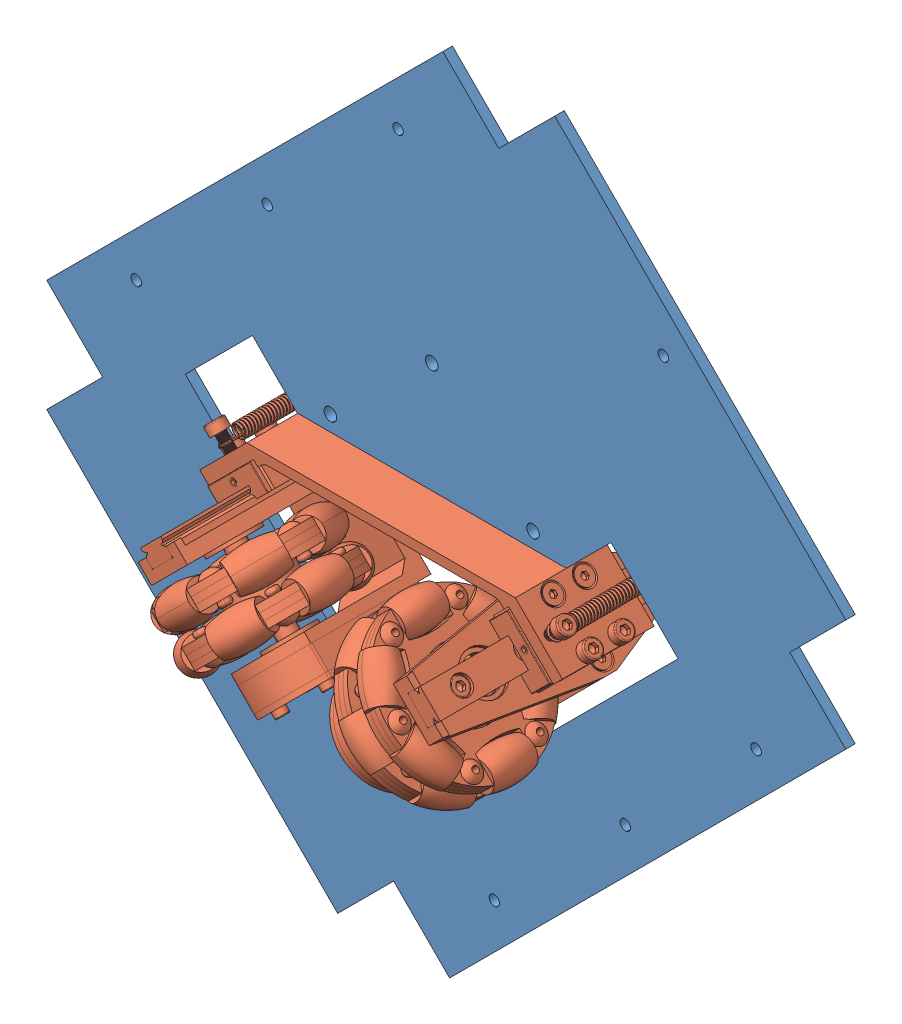
SolidWorks assembly 全局, configuration 默认. Lengths in mm.
Overall size (267.82 321.03 80.97).
2 component instances, 2 part files, 3 mates.
Components (placement in the parent):
- 全局定位固定板th 三代caijan-1: 全局定位固定板th 三代caijan [默认] at (-5.8748 -10.9195 319.5265) size (252.44 252.44 3)
- 东北大学全方位平面定位系统-1: 东北大学全方位平面定位系统 [默认] at (111.0335 85.0951 317.3519) x (0.707107 0.707107 0) z (0 0 1) size (104.96 104.71 80.97)
Mates (geometry in assembly coordinates):
- 同心1: concentric aligned: cylinder of 全局定位固定板th 三代caijan-1 through (-5.8748 88.9069 322.5265) axis (0 0 -1) radius 2; cylinder of 东北大学全方位平面定位系统-1 through (-5.8748 88.9069 319.5265) axis (0 0 -1) radius 2
- 重合1: coincident anti-aligned: plane of 全局定位固定板th 三代caijan-1 through (-5.8748 -10.9195 319.5265) normal (0 0 -1); plane of 东北大学全方位平面定位系统-1 through (-48.8103 53.9069 319.5265) normal (0 0 1)
- 同心2: concentric aligned: cylinder of 全局定位固定板th 三代caijan-1 through (26.1252 58.9069 322.5265) axis (0 0 -1) radius 2; cylinder of 东北大学全方位平面定位系统-1 through (26.1252 58.9069 319.5265) axis (0 0 -1) radius 2
